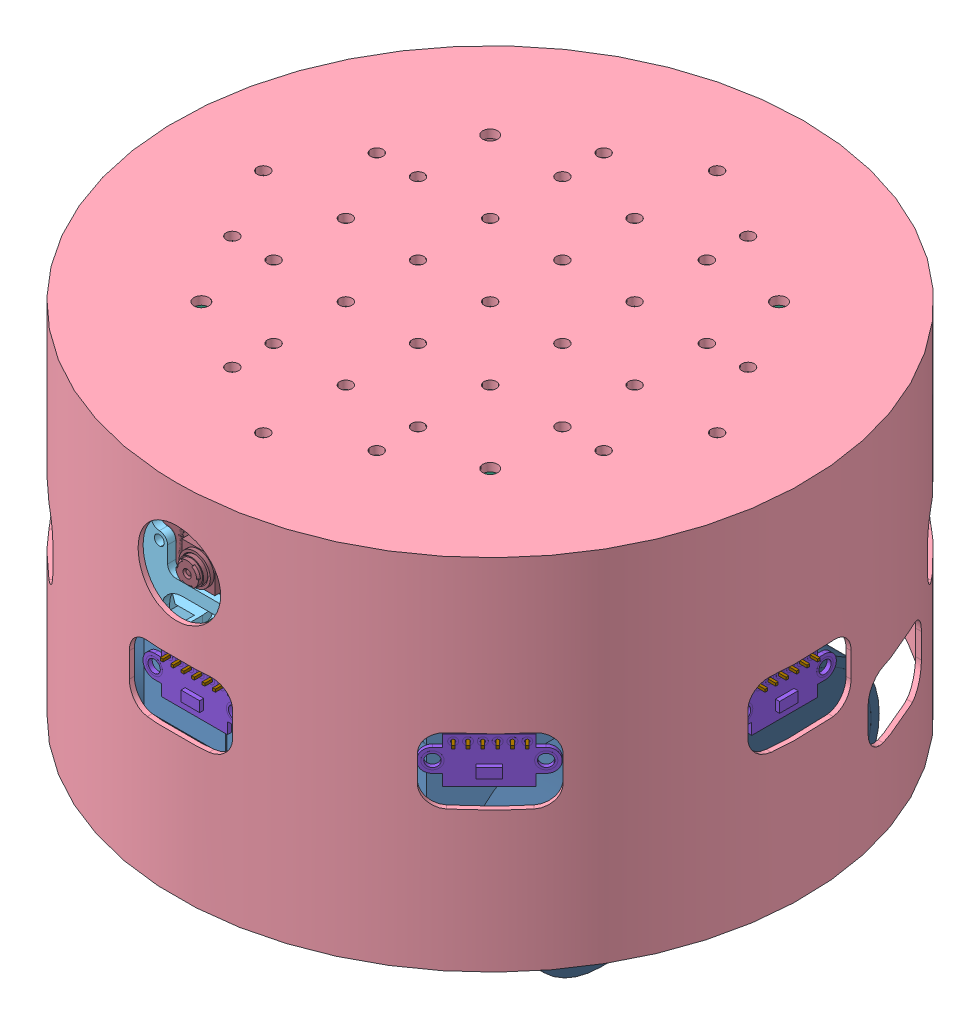
SolidWorks assembly affective_mobile_platform_ver_3, configuration Default. Lengths in mm.
Overall size (152 102.25 152).
598 component instances, 23 part files, 172 mates.
Components (placement in the parent):
- main_case-1: main_case [Default] at (56.0336 74.2064 51.1354) size (80.9 34.8 115.4)
- motor_holder-1: motor_holder [Default] at (56.0336 51.1064 74.8354) x (0 0 -1) z (-1 0 0) size (28 15 80.9)
- wheel_holder-1: wheel_holder [Default] at (74.0836 50.1064 122.8354) x (0 -1 0) z (0 0 1) size (14 20 27)
- wheel_holder-2: wheel_holder [Default] at (37.9836 50.1064 122.8354) x (0 -1 0) z (0 0 -1) size (14 20 27)
- power_bank-2: power_bank [Default] at (56.0336 72.6064 146.6354) x (-1 0 0) z (0 0 -1) size (66.5 23 95.6)
- 2nd_layer-1: 2nd_layer [Default] at (56.0336 89.3064 98.8354) size (130 1.6 130)
- H254_90deg_6pin-9: H254_90deg_6pin [Default] at (61.1135 93.4464 158.4354) x (-0.000003 0 1) z (1 -0.000004 0.000003) size (10.36 6.14 15.24)
  - H254_90deg_3pin-1: H254_90deg_3pin [Default] at origin size (10.36 6.14 7.62)
    - FrameAndPin_H254_90deg-1: FrameAndPin_H254_90deg [Default] at origin size (10.36 6.14 2.54)
      - frame_H254-1: frame_H254 [Default] at origin size (8.4 2.54 2.54)
      - pin-90deg-1: pin-90deg [Default] at (-0.0461 1.2682 1.27) x (0 0 -1) z (0.999998 -0.002105 0) size (1.95 5.07 7.58)
    - FrameAndPin_H254_90deg-2: FrameAndPin_H254_90deg [Default] at (0 0 -2.54) size (10.36 6.14 2.54)
      - frame_H254-1: frame_H254 [Default] at origin size (8.4 2.54 2.54)
      - pin-90deg-1: pin-90deg [Default] at (-0.0461 1.2682 1.27) x (0 0 -1) z (0.999998 -0.002105 0) size (1.95 5.07 7.58)
    - FrameAndPin_H254_90deg-4: FrameAndPin_H254_90deg [Default] at (0 0 -5.08) size (10.36 6.14 2.54)
      - frame_H254-1: frame_H254 [Default] at origin size (8.4 2.54 2.54)
      - pin-90deg-1: pin-90deg [Default] at (-0.0461 1.2682 1.27) x (0 0 -1) z (0.999998 -0.002105 0) size (1.95 5.07 7.58)
  - H254_90deg_3pin-2: H254_90deg_3pin [Default] at (0 0 -7.62) size (10.36 6.14 7.62)
    - FrameAndPin_H254_90deg-1: FrameAndPin_H254_90deg [Default] at origin size (10.36 6.14 2.54)
      - frame_H254-1: frame_H254 [Default] at origin size (8.4 2.54 2.54)
      - pin-90deg-1: pin-90deg [Default] at (-0.0461 1.2682 1.27) x (0 0 -1) z (0.999998 -0.002105 0) size (1.95 5.07 7.58)
    - FrameAndPin_H254_90deg-2: FrameAndPin_H254_90deg [Default] at (0 0 -2.54) size (10.36 6.14 2.54)
      - frame_H254-1: frame_H254 [Default] at origin size (8.4 2.54 2.54)
      - pin-90deg-1: pin-90deg [Default] at (-0.0461 1.2682 1.27) x (0 0 -1) z (0.999998 -0.002105 0) size (1.95 5.07 7.58)
    - FrameAndPin_H254_90deg-4: FrameAndPin_H254_90deg [Default] at (0 0 -5.08) size (10.36 6.14 2.54)
      - frame_H254-1: frame_H254 [Default] at origin size (8.4 2.54 2.54)
      - pin-90deg-1: pin-90deg [Default] at (-0.0461 1.2682 1.27) x (0 0 -1) z (0.999998 -0.002105 0) size (1.95 5.07 7.58)
- vl53l0x-9: vl53l0x [Default] at (55.8835 88.1764 169.3753) x (-1 0.000004 -0.000003) z (0.000004 1 0) size (25 11.3 11)
  - vl53l0x_PCB-1: vl53l0x_PCB [Default] at origin size (25 3 11)
  - pin_header-1: pin_header [Default] at (-6.5 -2.54 4) size (2.54 11.3 2.54)
  - pin_header-2: pin_header [Default] at (-3.96 -2.54 4) size (2.54 11.3 2.54)
  - pin_header-3: pin_header [Default] at (-1.42 -2.54 4) size (2.54 11.3 2.54)
  - pin_header-4: pin_header [Default] at (1.12 -2.54 4) size (2.54 11.3 2.54)
  - pin_header-5: pin_header [Default] at (3.66 -2.54 4) size (2.54 11.3 2.54)
  - pin_header-6: pin_header [Default] at (6.2 -2.54 4) size (2.54 11.3 2.54)
- wheels-1: wheels [Default] at (92.2336 51.1064 98.8354) x (0 0 -1) z (1 0 0) size (87 39 14.6)
- wheels-2: wheels [Default] at (19.8336 51.1064 98.8354) x (0 0 1) z (-1 0 0) size (87 39 14.6)
- spacer-2: spacer [Default] at (31.5336 90.9064 137.7975) x (0.77891 0 -0.627136) z (0.627136 0 0.77891) size (6.3 21 7.27)
- spacer-4: spacer [Default] at (80.5336 90.9064 79.7975) x (0 0 -1) z (1 0 0) size (6.3 21 7.27)
- spacer-5: spacer [Default] at (31.5336 90.9064 79.7975) x (0 0 1) z (-1 0 0) size (6.3 21 7.27)
- 1st_layer-1: 1st_layer [Default] at (37.9836 51.1064 122.8354) x (0 0 1) z (0 -1 0) size (65.3 46.5 2.57)
- vl53l0x-24: vl53l0x [Default] at (105.8067 88.1764 148.8208) x (-0.707109 0.000004 0.707104) z (0.000003 1 -0.000003) size (25 11.3 11)
  - vl53l0x_PCB-1: vl53l0x_PCB [Default] at origin size (25 3 11)
  - pin_header-1: pin_header [Default] at (-6.5 -2.54 4) size (2.54 11.3 2.54)
  - pin_header-2: pin_header [Default] at (-3.96 -2.54 4) size (2.54 11.3 2.54)
  - pin_header-3: pin_header [Default] at (-1.42 -2.54 4) size (2.54 11.3 2.54)
  - pin_header-4: pin_header [Default] at (1.12 -2.54 4) size (2.54 11.3 2.54)
  - pin_header-5: pin_header [Default] at (3.66 -2.54 4) size (2.54 11.3 2.54)
  - pin_header-6: pin_header [Default] at (6.2 -2.54 4) size (2.54 11.3 2.54)
- vl53l0x-25: vl53l0x [Default] at (126.5735 88.1764 98.9854) x (-0.000003 0.000004 1) z (0 1 -0.000004) size (25 11.3 11)
  - vl53l0x_PCB-1: vl53l0x_PCB [Default] at origin size (25 3 11)
  - pin_header-1: pin_header [Default] at (-6.5 -2.54 4) size (2.54 11.3 2.54)
  - pin_header-2: pin_header [Default] at (-3.96 -2.54 4) size (2.54 11.3 2.54)
  - pin_header-3: pin_header [Default] at (-1.42 -2.54 4) size (2.54 11.3 2.54)
  - pin_header-4: pin_header [Default] at (1.12 -2.54 4) size (2.54 11.3 2.54)
  - pin_header-5: pin_header [Default] at (3.66 -2.54 4) size (2.54 11.3 2.54)
  - pin_header-6: pin_header [Default] at (6.2 -2.54 4) size (2.54 11.3 2.54)
- vl53l0x-26: vl53l0x [Default] at (106.019 88.1764 49.0622) x (0.707104 0.000004 0.707109) z (-0.000003 1 -0.000003) size (25 11.3 11)
  - vl53l0x_PCB-1: vl53l0x_PCB [Default] at origin size (25 3 11)
  - pin_header-1: pin_header [Default] at (-6.5 -2.54 4) size (2.54 11.3 2.54)
  - pin_header-2: pin_header [Default] at (-3.96 -2.54 4) size (2.54 11.3 2.54)
  - pin_header-3: pin_header [Default] at (-1.42 -2.54 4) size (2.54 11.3 2.54)
  - pin_header-4: pin_header [Default] at (1.12 -2.54 4) size (2.54 11.3 2.54)
  - pin_header-5: pin_header [Default] at (3.66 -2.54 4) size (2.54 11.3 2.54)
  - pin_header-6: pin_header [Default] at (6.2 -2.54 4) size (2.54 11.3 2.54)
- vl53l0x-27: vl53l0x [Default] at (56.1836 88.1764 28.2954) x (1 0.000004 0.000003) z (-0.000004 1 0) size (25 11.3 11)
  - vl53l0x_PCB-1: vl53l0x_PCB [Default] at origin size (25 3 11)
  - pin_header-1: pin_header [Default] at (-6.5 -2.54 4) size (2.54 11.3 2.54)
  - pin_header-2: pin_header [Default] at (-3.96 -2.54 4) size (2.54 11.3 2.54)
  - pin_header-3: pin_header [Default] at (-1.42 -2.54 4) size (2.54 11.3 2.54)
  - pin_header-4: pin_header [Default] at (1.12 -2.54 4) size (2.54 11.3 2.54)
  - pin_header-5: pin_header [Default] at (3.66 -2.54 4) size (2.54 11.3 2.54)
  - pin_header-6: pin_header [Default] at (6.2 -2.54 4) size (2.54 11.3 2.54)
- vl53l0x-28: vl53l0x [Default] at (6.2604 88.1764 48.85) x (0.707109 0.000004 -0.707104) z (-0.000003 1 0.000003) size (25 11.3 11)
  - vl53l0x_PCB-1: vl53l0x_PCB [Default] at origin size (25 3 11)
  - pin_header-1: pin_header [Default] at (-6.5 -2.54 4) size (2.54 11.3 2.54)
  - pin_header-2: pin_header [Default] at (-3.96 -2.54 4) size (2.54 11.3 2.54)
  - pin_header-3: pin_header [Default] at (-1.42 -2.54 4) size (2.54 11.3 2.54)
  - pin_header-4: pin_header [Default] at (1.12 -2.54 4) size (2.54 11.3 2.54)
  - pin_header-5: pin_header [Default] at (3.66 -2.54 4) size (2.54 11.3 2.54)
  - pin_header-6: pin_header [Default] at (6.2 -2.54 4) size (2.54 11.3 2.54)
- vl53l0x-29: vl53l0x [Default] at (-14.5064 88.1764 98.6853) x (0.000003 0.000004 -1) z (0 1 0.000004) size (25 11.3 11)
  - vl53l0x_PCB-1: vl53l0x_PCB [Default] at origin size (25 3 11)
  - pin_header-1: pin_header [Default] at (-6.5 -2.54 4) size (2.54 11.3 2.54)
  - pin_header-2: pin_header [Default] at (-3.96 -2.54 4) size (2.54 11.3 2.54)
  - pin_header-3: pin_header [Default] at (-1.42 -2.54 4) size (2.54 11.3 2.54)
  - pin_header-4: pin_header [Default] at (1.12 -2.54 4) size (2.54 11.3 2.54)
  - pin_header-5: pin_header [Default] at (3.66 -2.54 4) size (2.54 11.3 2.54)
  - pin_header-6: pin_header [Default] at (6.2 -2.54 4) size (2.54 11.3 2.54)
- vl53l0x-30: vl53l0x [Default] at (6.0481 88.1764 148.6086) x (-0.707104 0.000004 -0.707109) z (0.000003 1 0.000003) size (25 11.3 11)
  - vl53l0x_PCB-1: vl53l0x_PCB [Default] at origin size (25 3 11)
  - pin_header-1: pin_header [Default] at (-6.5 -2.54 4) size (2.54 11.3 2.54)
  - pin_header-2: pin_header [Default] at (-3.96 -2.54 4) size (2.54 11.3 2.54)
  - pin_header-3: pin_header [Default] at (-1.42 -2.54 4) size (2.54 11.3 2.54)
  - pin_header-4: pin_header [Default] at (1.12 -2.54 4) size (2.54 11.3 2.54)
  - pin_header-5: pin_header [Default] at (3.66 -2.54 4) size (2.54 11.3 2.54)
  - pin_header-6: pin_header [Default] at (6.2 -2.54 4) size (2.54 11.3 2.54)
- H254_90deg_6pin-24: H254_90deg_6pin [Default] at (101.7692 93.4464 137.3868) x (0.707104 0 0.707109) z (0.707109 -0.000004 -0.707104) size (10.36 6.14 15.24)
  - H254_90deg_3pin-1: H254_90deg_3pin [Default] at origin size (10.36 6.14 7.62)
    - FrameAndPin_H254_90deg-1: FrameAndPin_H254_90deg [Default] at origin size (10.36 6.14 2.54)
      - frame_H254-1: frame_H254 [Default] at origin size (8.4 2.54 2.54)
      - pin-90deg-1: pin-90deg [Default] at (-0.0461 1.2682 1.27) x (0 0 -1) z (0.999998 -0.002105 0) size (1.95 5.07 7.58)
    - FrameAndPin_H254_90deg-2: FrameAndPin_H254_90deg [Default] at (0 0 -2.54) size (10.36 6.14 2.54)
      - frame_H254-1: frame_H254 [Default] at origin size (8.4 2.54 2.54)
      - pin-90deg-1: pin-90deg [Default] at (-0.0461 1.2682 1.27) x (0 0 -1) z (0.999998 -0.002105 0) size (1.95 5.07 7.58)
    - FrameAndPin_H254_90deg-4: FrameAndPin_H254_90deg [Default] at (0 0 -5.08) size (10.36 6.14 2.54)
      - frame_H254-1: frame_H254 [Default] at origin size (8.4 2.54 2.54)
      - pin-90deg-1: pin-90deg [Default] at (-0.0461 1.2682 1.27) x (0 0 -1) z (0.999998 -0.002105 0) size (1.95 5.07 7.58)
  - H254_90deg_3pin-2: H254_90deg_3pin [Default] at (0 0 -7.62) size (10.36 6.14 7.62)
    - FrameAndPin_H254_90deg-1: FrameAndPin_H254_90deg [Default] at origin size (10.36 6.14 2.54)
      - frame_H254-1: frame_H254 [Default] at origin size (8.4 2.54 2.54)
      - pin-90deg-1: pin-90deg [Default] at (-0.0461 1.2682 1.27) x (0 0 -1) z (0.999998 -0.002105 0) size (1.95 5.07 7.58)
    - FrameAndPin_H254_90deg-2: FrameAndPin_H254_90deg [Default] at (0 0 -2.54) size (10.36 6.14 2.54)
      - frame_H254-1: frame_H254 [Default] at origin size (8.4 2.54 2.54)
      - pin-90deg-1: pin-90deg [Default] at (-0.0461 1.2682 1.27) x (0 0 -1) z (0.999998 -0.002105 0) size (1.95 5.07 7.58)
    - FrameAndPin_H254_90deg-4: FrameAndPin_H254_90deg [Default] at (0 0 -5.08) size (10.36 6.14 2.54)
      - frame_H254-1: frame_H254 [Default] at origin size (8.4 2.54 2.54)
      - pin-90deg-1: pin-90deg [Default] at (-0.0461 1.2682 1.27) x (0 0 -1) z (0.999998 -0.002105 0) size (1.95 5.07 7.58)
- H254_90deg_6pin-25: H254_90deg_6pin [Default] at (115.6336 93.4464 93.7554) x (1 0 0.000003) z (0.000003 -0.000004 -1) size (10.36 6.14 15.24)
  - H254_90deg_3pin-1: H254_90deg_3pin [Default] at origin size (10.36 6.14 7.62)
    - FrameAndPin_H254_90deg-1: FrameAndPin_H254_90deg [Default] at origin size (10.36 6.14 2.54)
      - frame_H254-1: frame_H254 [Default] at origin size (8.4 2.54 2.54)
      - pin-90deg-1: pin-90deg [Default] at (-0.0461 1.2682 1.27) x (0 0 -1) z (0.999998 -0.002105 0) size (1.95 5.07 7.58)
    - FrameAndPin_H254_90deg-2: FrameAndPin_H254_90deg [Default] at (0 0 -2.54) size (10.36 6.14 2.54)
      - frame_H254-1: frame_H254 [Default] at origin size (8.4 2.54 2.54)
      - pin-90deg-1: pin-90deg [Default] at (-0.0461 1.2682 1.27) x (0 0 -1) z (0.999998 -0.002105 0) size (1.95 5.07 7.58)
    - FrameAndPin_H254_90deg-4: FrameAndPin_H254_90deg [Default] at (0 0 -5.08) size (10.36 6.14 2.54)
      - frame_H254-1: frame_H254 [Default] at origin size (8.4 2.54 2.54)
      - pin-90deg-1: pin-90deg [Default] at (-0.0461 1.2682 1.27) x (0 0 -1) z (0.999998 -0.002105 0) size (1.95 5.07 7.58)
  - H254_90deg_3pin-2: H254_90deg_3pin [Default] at (0 0 -7.62) size (10.36 6.14 7.62)
    - FrameAndPin_H254_90deg-1: FrameAndPin_H254_90deg [Default] at origin size (10.36 6.14 2.54)
      - frame_H254-1: frame_H254 [Default] at origin size (8.4 2.54 2.54)
      - pin-90deg-1: pin-90deg [Default] at (-0.0461 1.2682 1.27) x (0 0 -1) z (0.999998 -0.002105 0) size (1.95 5.07 7.58)
    - FrameAndPin_H254_90deg-2: FrameAndPin_H254_90deg [Default] at (0 0 -2.54) size (10.36 6.14 2.54)
      - frame_H254-1: frame_H254 [Default] at origin size (8.4 2.54 2.54)
      - pin-90deg-1: pin-90deg [Default] at (-0.0461 1.2682 1.27) x (0 0 -1) z (0.999998 -0.002105 0) size (1.95 5.07 7.58)
    - FrameAndPin_H254_90deg-4: FrameAndPin_H254_90deg [Default] at (0 0 -5.08) size (10.36 6.14 2.54)
      - frame_H254-1: frame_H254 [Default] at origin size (8.4 2.54 2.54)
      - pin-90deg-1: pin-90deg [Default] at (-0.0461 1.2682 1.27) x (0 0 -1) z (0.999998 -0.002105 0) size (1.95 5.07 7.58)
- H254_90deg_6pin-26: H254_90deg_6pin [Default] at (94.585 93.4464 53.0997) x (0.707109 0 -0.707104) z (-0.707104 -0.000004 -0.707109) size (10.36 6.14 15.24)
  - H254_90deg_3pin-1: H254_90deg_3pin [Default] at origin size (10.36 6.14 7.62)
    - FrameAndPin_H254_90deg-1: FrameAndPin_H254_90deg [Default] at origin size (10.36 6.14 2.54)
      - frame_H254-1: frame_H254 [Default] at origin size (8.4 2.54 2.54)
      - pin-90deg-1: pin-90deg [Default] at (-0.0461 1.2682 1.27) x (0 0 -1) z (0.999998 -0.002105 0) size (1.95 5.07 7.58)
    - FrameAndPin_H254_90deg-2: FrameAndPin_H254_90deg [Default] at (0 0 -2.54) size (10.36 6.14 2.54)
      - frame_H254-1: frame_H254 [Default] at origin size (8.4 2.54 2.54)
      - pin-90deg-1: pin-90deg [Default] at (-0.0461 1.2682 1.27) x (0 0 -1) z (0.999998 -0.002105 0) size (1.95 5.07 7.58)
    - FrameAndPin_H254_90deg-4: FrameAndPin_H254_90deg [Default] at (0 0 -5.08) size (10.36 6.14 2.54)
      - frame_H254-1: frame_H254 [Default] at origin size (8.4 2.54 2.54)
      - pin-90deg-1: pin-90deg [Default] at (-0.0461 1.2682 1.27) x (0 0 -1) z (0.999998 -0.002105 0) size (1.95 5.07 7.58)
  - H254_90deg_3pin-2: H254_90deg_3pin [Default] at (0 0 -7.62) size (10.36 6.14 7.62)
    - FrameAndPin_H254_90deg-1: FrameAndPin_H254_90deg [Default] at origin size (10.36 6.14 2.54)
      - frame_H254-1: frame_H254 [Default] at origin size (8.4 2.54 2.54)
      - pin-90deg-1: pin-90deg [Default] at (-0.0461 1.2682 1.27) x (0 0 -1) z (0.999998 -0.002105 0) size (1.95 5.07 7.58)
    - FrameAndPin_H254_90deg-2: FrameAndPin_H254_90deg [Default] at (0 0 -2.54) size (10.36 6.14 2.54)
      - frame_H254-1: frame_H254 [Default] at origin size (8.4 2.54 2.54)
      - pin-90deg-1: pin-90deg [Default] at (-0.0461 1.2682 1.27) x (0 0 -1) z (0.999998 -0.002105 0) size (1.95 5.07 7.58)
    - FrameAndPin_H254_90deg-4: FrameAndPin_H254_90deg [Default] at (0 0 -5.08) size (10.36 6.14 2.54)
      - frame_H254-1: frame_H254 [Default] at origin size (8.4 2.54 2.54)
      - pin-90deg-1: pin-90deg [Default] at (-0.0461 1.2682 1.27) x (0 0 -1) z (0.999998 -0.002105 0) size (1.95 5.07 7.58)
- H254_90deg_6pin-27: H254_90deg_6pin [Default] at (50.9536 93.4464 39.2354) x (0.000003 0 -1) z (-1 -0.000004 -0.000003) size (10.36 6.14 15.24)
  - H254_90deg_3pin-1: H254_90deg_3pin [Default] at origin size (10.36 6.14 7.62)
    - FrameAndPin_H254_90deg-1: FrameAndPin_H254_90deg [Default] at origin size (10.36 6.14 2.54)
      - frame_H254-1: frame_H254 [Default] at origin size (8.4 2.54 2.54)
      - pin-90deg-1: pin-90deg [Default] at (-0.0461 1.2682 1.27) x (0 0 -1) z (0.999998 -0.002105 0) size (1.95 5.07 7.58)
    - FrameAndPin_H254_90deg-2: FrameAndPin_H254_90deg [Default] at (0 0 -2.54) size (10.36 6.14 2.54)
      - frame_H254-1: frame_H254 [Default] at origin size (8.4 2.54 2.54)
      - pin-90deg-1: pin-90deg [Default] at (-0.0461 1.2682 1.27) x (0 0 -1) z (0.999998 -0.002105 0) size (1.95 5.07 7.58)
    - FrameAndPin_H254_90deg-4: FrameAndPin_H254_90deg [Default] at (0 0 -5.08) size (10.36 6.14 2.54)
      - frame_H254-1: frame_H254 [Default] at origin size (8.4 2.54 2.54)
      - pin-90deg-1: pin-90deg [Default] at (-0.0461 1.2682 1.27) x (0 0 -1) z (0.999998 -0.002105 0) size (1.95 5.07 7.58)
  - H254_90deg_3pin-2: H254_90deg_3pin [Default] at (0 0 -7.62) size (10.36 6.14 7.62)
    - FrameAndPin_H254_90deg-1: FrameAndPin_H254_90deg [Default] at origin size (10.36 6.14 2.54)
      - frame_H254-1: frame_H254 [Default] at origin size (8.4 2.54 2.54)
      - pin-90deg-1: pin-90deg [Default] at (-0.0461 1.2682 1.27) x (0 0 -1) z (0.999998 -0.002105 0) size (1.95 5.07 7.58)
    - FrameAndPin_H254_90deg-2: FrameAndPin_H254_90deg [Default] at (0 0 -2.54) size (10.36 6.14 2.54)
      - frame_H254-1: frame_H254 [Default] at origin size (8.4 2.54 2.54)
      - pin-90deg-1: pin-90deg [Default] at (-0.0461 1.2682 1.27) x (0 0 -1) z (0.999998 -0.002105 0) size (1.95 5.07 7.58)
    - FrameAndPin_H254_90deg-4: FrameAndPin_H254_90deg [Default] at (0 0 -5.08) size (10.36 6.14 2.54)
      - frame_H254-1: frame_H254 [Default] at origin size (8.4 2.54 2.54)
      - pin-90deg-1: pin-90deg [Default] at (-0.0461 1.2682 1.27) x (0 0 -1) z (0.999998 -0.002105 0) size (1.95 5.07 7.58)
- H254_90deg_6pin-28: H254_90deg_6pin [Default] at (10.2979 93.4464 60.2839) x (-0.707104 0 -0.707109) z (-0.707109 -0.000004 0.707104) size (10.36 6.14 15.24)
  - H254_90deg_3pin-1: H254_90deg_3pin [Default] at origin size (10.36 6.14 7.62)
    - FrameAndPin_H254_90deg-1: FrameAndPin_H254_90deg [Default] at origin size (10.36 6.14 2.54)
      - frame_H254-1: frame_H254 [Default] at origin size (8.4 2.54 2.54)
      - pin-90deg-1: pin-90deg [Default] at (-0.0461 1.2682 1.27) x (0 0 -1) z (0.999998 -0.002105 0) size (1.95 5.07 7.58)
    - FrameAndPin_H254_90deg-2: FrameAndPin_H254_90deg [Default] at (0 0 -2.54) size (10.36 6.14 2.54)
      - frame_H254-1: frame_H254 [Default] at origin size (8.4 2.54 2.54)
      - pin-90deg-1: pin-90deg [Default] at (-0.0461 1.2682 1.27) x (0 0 -1) z (0.999998 -0.002105 0) size (1.95 5.07 7.58)
    - FrameAndPin_H254_90deg-4: FrameAndPin_H254_90deg [Default] at (0 0 -5.08) size (10.36 6.14 2.54)
      - frame_H254-1: frame_H254 [Default] at origin size (8.4 2.54 2.54)
      - pin-90deg-1: pin-90deg [Default] at (-0.0461 1.2682 1.27) x (0 0 -1) z (0.999998 -0.002105 0) size (1.95 5.07 7.58)
  - H254_90deg_3pin-2: H254_90deg_3pin [Default] at (0 0 -7.62) size (10.36 6.14 7.62)
    - FrameAndPin_H254_90deg-1: FrameAndPin_H254_90deg [Default] at origin size (10.36 6.14 2.54)
      - frame_H254-1: frame_H254 [Default] at origin size (8.4 2.54 2.54)
      - pin-90deg-1: pin-90deg [Default] at (-0.0461 1.2682 1.27) x (0 0 -1) z (0.999998 -0.002105 0) size (1.95 5.07 7.58)
    - FrameAndPin_H254_90deg-2: FrameAndPin_H254_90deg [Default] at (0 0 -2.54) size (10.36 6.14 2.54)
      - frame_H254-1: frame_H254 [Default] at origin size (8.4 2.54 2.54)
      - pin-90deg-1: pin-90deg [Default] at (-0.0461 1.2682 1.27) x (0 0 -1) z (0.999998 -0.002105 0) size (1.95 5.07 7.58)
    - FrameAndPin_H254_90deg-4: FrameAndPin_H254_90deg [Default] at (0 0 -5.08) size (10.36 6.14 2.54)
      - frame_H254-1: frame_H254 [Default] at origin size (8.4 2.54 2.54)
      - pin-90deg-1: pin-90deg [Default] at (-0.0461 1.2682 1.27) x (0 0 -1) z (0.999998 -0.002105 0) size (1.95 5.07 7.58)
- H254_90deg_6pin-29: H254_90deg_6pin [Default] at (-3.5664 93.4464 103.9154) x (-1 0 -0.000003) z (-0.000003 -0.000004 1) size (10.36 6.14 15.24)
  - H254_90deg_3pin-1: H254_90deg_3pin [Default] at origin size (10.36 6.14 7.62)
    - FrameAndPin_H254_90deg-1: FrameAndPin_H254_90deg [Default] at origin size (10.36 6.14 2.54)
      - frame_H254-1: frame_H254 [Default] at origin size (8.4 2.54 2.54)
      - pin-90deg-1: pin-90deg [Default] at (-0.0461 1.2682 1.27) x (0 0 -1) z (0.999998 -0.002105 0) size (1.95 5.07 7.58)
    - FrameAndPin_H254_90deg-2: FrameAndPin_H254_90deg [Default] at (0 0 -2.54) size (10.36 6.14 2.54)
      - frame_H254-1: frame_H254 [Default] at origin size (8.4 2.54 2.54)
      - pin-90deg-1: pin-90deg [Default] at (-0.0461 1.2682 1.27) x (0 0 -1) z (0.999998 -0.002105 0) size (1.95 5.07 7.58)
    - FrameAndPin_H254_90deg-4: FrameAndPin_H254_90deg [Default] at (0 0 -5.08) size (10.36 6.14 2.54)
      - frame_H254-1: frame_H254 [Default] at origin size (8.4 2.54 2.54)
      - pin-90deg-1: pin-90deg [Default] at (-0.0461 1.2682 1.27) x (0 0 -1) z (0.999998 -0.002105 0) size (1.95 5.07 7.58)
  - H254_90deg_3pin-2: H254_90deg_3pin [Default] at (0 0 -7.62) size (10.36 6.14 7.62)
    - FrameAndPin_H254_90deg-1: FrameAndPin_H254_90deg [Default] at origin size (10.36 6.14 2.54)
      - frame_H254-1: frame_H254 [Default] at origin size (8.4 2.54 2.54)
      - pin-90deg-1: pin-90deg [Default] at (-0.0461 1.2682 1.27) x (0 0 -1) z (0.999998 -0.002105 0) size (1.95 5.07 7.58)
    - FrameAndPin_H254_90deg-2: FrameAndPin_H254_90deg [Default] at (0 0 -2.54) size (10.36 6.14 2.54)
      - frame_H254-1: frame_H254 [Default] at origin size (8.4 2.54 2.54)
      - pin-90deg-1: pin-90deg [Default] at (-0.0461 1.2682 1.27) x (0 0 -1) z (0.999998 -0.002105 0) size (1.95 5.07 7.58)
    - FrameAndPin_H254_90deg-4: FrameAndPin_H254_90deg [Default] at (0 0 -5.08) size (10.36 6.14 2.54)
      - frame_H254-1: frame_H254 [Default] at origin size (8.4 2.54 2.54)
      - pin-90deg-1: pin-90deg [Default] at (-0.0461 1.2682 1.27) x (0 0 -1) z (0.999998 -0.002105 0) size (1.95 5.07 7.58)
- H254_90deg_6pin-30: H254_90deg_6pin [Default] at (17.4821 93.4464 144.571) x (-0.707109 0 0.707104) z (0.707104 -0.000004 0.707109) size (10.36 6.14 15.24)
  - H254_90deg_3pin-1: H254_90deg_3pin [Default] at origin size (10.36 6.14 7.62)
    - FrameAndPin_H254_90deg-1: FrameAndPin_H254_90deg [Default] at origin size (10.36 6.14 2.54)
      - frame_H254-1: frame_H254 [Default] at origin size (8.4 2.54 2.54)
      - pin-90deg-1: pin-90deg [Default] at (-0.0461 1.2682 1.27) x (0 0 -1) z (0.999998 -0.002105 0) size (1.95 5.07 7.58)
    - FrameAndPin_H254_90deg-2: FrameAndPin_H254_90deg [Default] at (0 0 -2.54) size (10.36 6.14 2.54)
      - frame_H254-1: frame_H254 [Default] at origin size (8.4 2.54 2.54)
      - pin-90deg-1: pin-90deg [Default] at (-0.0461 1.2682 1.27) x (0 0 -1) z (0.999998 -0.002105 0) size (1.95 5.07 7.58)
    - FrameAndPin_H254_90deg-4: FrameAndPin_H254_90deg [Default] at (0 0 -5.08) size (10.36 6.14 2.54)
      - frame_H254-1: frame_H254 [Default] at origin size (8.4 2.54 2.54)
      - pin-90deg-1: pin-90deg [Default] at (-0.0461 1.2682 1.27) x (0 0 -1) z (0.999998 -0.002105 0) size (1.95 5.07 7.58)
  - H254_90deg_3pin-2: H254_90deg_3pin [Default] at (0 0 -7.62) size (10.36 6.14 7.62)
    - FrameAndPin_H254_90deg-1: FrameAndPin_H254_90deg [Default] at origin size (10.36 6.14 2.54)
      - frame_H254-1: frame_H254 [Default] at origin size (8.4 2.54 2.54)
      - pin-90deg-1: pin-90deg [Default] at (-0.0461 1.2682 1.27) x (0 0 -1) z (0.999998 -0.002105 0) size (1.95 5.07 7.58)
    - FrameAndPin_H254_90deg-2: FrameAndPin_H254_90deg [Default] at (0 0 -2.54) size (10.36 6.14 2.54)
      - frame_H254-1: frame_H254 [Default] at origin size (8.4 2.54 2.54)
      - pin-90deg-1: pin-90deg [Default] at (-0.0461 1.2682 1.27) x (0 0 -1) z (0.999998 -0.002105 0) size (1.95 5.07 7.58)
    - FrameAndPin_H254_90deg-4: FrameAndPin_H254_90deg [Default] at (0 0 -5.08) size (10.36 6.14 2.54)
      - frame_H254-1: frame_H254 [Default] at origin size (8.4 2.54 2.54)
      - pin-90deg-1: pin-90deg [Default] at (-0.0461 1.2682 1.27) x (0 0 -1) z (0.999998 -0.002105 0) size (1.95 5.07 7.58)
- camera-1: camera [Default] at (56.1278 115.9111 165.5354) x (0 1 0) z (0 0 1) size (23.86 25 9.96)
- raspberryPi3B-1: raspberryPi3B [Detailed] at (56.0336 107.2064 98.7975) x (0 0 -1) z (0 -1 0) size (87.05 58.5 19.05)
- spacer-8: spacer [Default] at (80.5336 90.9064 137.7975) x (0.77891 0 -0.627136) z (0.627136 0 0.77891) size (6.3 21 7.27)
- 3rd_layer-1: 3rd_layer [Default] at (56.0336 115.2592 98.8354) x (-1 0 0) z (0 1 0) size (130 109 1.6)
- Header_1x20pin-1: Header_1x20pin [Default] at (105.5636 90.9064 122.1244) size (2.54 10.59 50.8)
  - header-1: header [Default] at origin size (2.54 10.59 2.54)
    - header-1: header [Default] at origin size (2.54 8.5 2.54)
    - pin-1: pin [Default] at (-1.4 0 0) size (0.4 10 1.99)
  - header-2: header [Default] at (0 0 -2.54) size (2.54 10.59 2.54)
    - header-1: header [Default] at origin size (2.54 8.5 2.54)
    - pin-1: pin [Default] at (-1.4 0 0) size (0.4 10 1.99)
  - header-3: header [Default] at (0 0 -5.08) size (2.54 10.59 2.54)
    - header-1: header [Default] at origin size (2.54 8.5 2.54)
    - pin-1: pin [Default] at (-1.4 0 0) size (0.4 10 1.99)
  - header-4: header [Default] at (0 0 -7.62) size (2.54 10.59 2.54)
    - header-1: header [Default] at origin size (2.54 8.5 2.54)
    - pin-1: pin [Default] at (-1.4 0 0) size (0.4 10 1.99)
  - header-5: header [Default] at (0 0 -10.16) size (2.54 10.59 2.54)
    - header-1: header [Default] at origin size (2.54 8.5 2.54)
    - pin-1: pin [Default] at (-1.4 0 0) size (0.4 10 1.99)
  - header-6: header [Default] at (0 0 -12.7) size (2.54 10.59 2.54)
    - header-1: header [Default] at origin size (2.54 8.5 2.54)
    - pin-1: pin [Default] at (-1.4 0 0) size (0.4 10 1.99)
  - header-7: header [Default] at (0 0 -15.24) size (2.54 10.59 2.54)
    - header-1: header [Default] at origin size (2.54 8.5 2.54)
    - pin-1: pin [Default] at (-1.4 0 0) size (0.4 10 1.99)
  - header-8: header [Default] at (0 0 -17.78) size (2.54 10.59 2.54)
    - header-1: header [Default] at origin size (2.54 8.5 2.54)
    - pin-1: pin [Default] at (-1.4 0 0) size (0.4 10 1.99)
  - header-9: header [Default] at (0 0 -20.32) size (2.54 10.59 2.54)
    - header-1: header [Default] at origin size (2.54 8.5 2.54)
    - pin-1: pin [Default] at (-1.4 0 0) size (0.4 10 1.99)
  - header-10: header [Default] at (0 0 -22.86) size (2.54 10.59 2.54)
    - header-1: header [Default] at origin size (2.54 8.5 2.54)
    - pin-1: pin [Default] at (-1.4 0 0) size (0.4 10 1.99)
  - header-11: header [Default] at (0 0 -25.4) size (2.54 10.59 2.54)
    - header-1: header [Default] at origin size (2.54 8.5 2.54)
    - pin-1: pin [Default] at (-1.4 0 0) size (0.4 10 1.99)
  - header-12: header [Default] at (0 0 -27.94) size (2.54 10.59 2.54)
    - header-1: header [Default] at origin size (2.54 8.5 2.54)
    - pin-1: pin [Default] at (-1.4 0 0) size (0.4 10 1.99)
  - header-13: header [Default] at (0 0 -30.48) size (2.54 10.59 2.54)
    - header-1: header [Default] at origin size (2.54 8.5 2.54)
    - pin-1: pin [Default] at (-1.4 0 0) size (0.4 10 1.99)
  - header-14: header [Default] at (0 0 -33.02) size (2.54 10.59 2.54)
    - header-1: header [Default] at origin size (2.54 8.5 2.54)
    - pin-1: pin [Default] at (-1.4 0 0) size (0.4 10 1.99)
  - header-15: header [Default] at (0 0 -35.56) size (2.54 10.59 2.54)
    - header-1: header [Default] at origin size (2.54 8.5 2.54)
    - pin-1: pin [Default] at (-1.4 0 0) size (0.4 10 1.99)
  - header-16: header [Default] at (0 0 -38.1) size (2.54 10.59 2.54)
    - header-1: header [Default] at origin size (2.54 8.5 2.54)
    - pin-1: pin [Default] at (-1.4 0 0) size (0.4 10 1.99)
  - header-17: header [Default] at (0 0 -40.64) size (2.54 10.59 2.54)
    - header-1: header [Default] at origin size (2.54 8.5 2.54)
    - pin-1: pin [Default] at (-1.4 0 0) size (0.4 10 1.99)
  - header-18: header [Default] at (0 0 -43.18) size (2.54 10.59 2.54)
    - header-1: header [Default] at origin size (2.54 8.5 2.54)
    - pin-1: pin [Default] at (-1.4 0 0) size (0.4 10 1.99)
  - header-19: header [Default] at (0 0 -45.72) size (2.54 10.59 2.54)
    - header-1: header [Default] at origin size (2.54 8.5 2.54)
    - pin-1: pin [Default] at (-1.4 0 0) size (0.4 10 1.99)
  - header-20: header [Default] at (0 0 -48.26) size (2.54 10.59 2.54)
    - header-1: header [Default] at origin size (2.54 8.5 2.54)
    - pin-1: pin [Default] at (-1.4 0 0) size (0.4 10 1.99)
- Header_1x20pin-2: Header_1x20pin [Default] at (9.0436 90.9064 122.1244) size (2.54 10.59 50.8)
  - header-1: header [Default] at origin size (2.54 10.59 2.54)
    - header-1: header [Default] at origin size (2.54 8.5 2.54)
    - pin-1: pin [Default] at (-1.4 0 0) size (0.4 10 1.99)
  - header-2: header [Default] at (0 0 -2.54) size (2.54 10.59 2.54)
    - header-1: header [Default] at origin size (2.54 8.5 2.54)
    - pin-1: pin [Default] at (-1.4 0 0) size (0.4 10 1.99)
  - header-3: header [Default] at (0 0 -5.08) size (2.54 10.59 2.54)
    - header-1: header [Default] at origin size (2.54 8.5 2.54)
    - pin-1: pin [Default] at (-1.4 0 0) size (0.4 10 1.99)
  - header-4: header [Default] at (0 0 -7.62) size (2.54 10.59 2.54)
    - header-1: header [Default] at origin size (2.54 8.5 2.54)
    - pin-1: pin [Default] at (-1.4 0 0) size (0.4 10 1.99)
  - header-5: header [Default] at (0 0 -10.16) size (2.54 10.59 2.54)
    - header-1: header [Default] at origin size (2.54 8.5 2.54)
    - pin-1: pin [Default] at (-1.4 0 0) size (0.4 10 1.99)
  - header-6: header [Default] at (0 0 -12.7) size (2.54 10.59 2.54)
    - header-1: header [Default] at origin size (2.54 8.5 2.54)
    - pin-1: pin [Default] at (-1.4 0 0) size (0.4 10 1.99)
  - header-7: header [Default] at (0 0 -15.24) size (2.54 10.59 2.54)
    - header-1: header [Default] at origin size (2.54 8.5 2.54)
    - pin-1: pin [Default] at (-1.4 0 0) size (0.4 10 1.99)
  - header-8: header [Default] at (0 0 -17.78) size (2.54 10.59 2.54)
    - header-1: header [Default] at origin size (2.54 8.5 2.54)
    - pin-1: pin [Default] at (-1.4 0 0) size (0.4 10 1.99)
  - header-9: header [Default] at (0 0 -20.32) size (2.54 10.59 2.54)
    - header-1: header [Default] at origin size (2.54 8.5 2.54)
    - pin-1: pin [Default] at (-1.4 0 0) size (0.4 10 1.99)
  - header-10: header [Default] at (0 0 -22.86) size (2.54 10.59 2.54)
    - header-1: header [Default] at origin size (2.54 8.5 2.54)
    - pin-1: pin [Default] at (-1.4 0 0) size (0.4 10 1.99)
  - header-11: header [Default] at (0 0 -25.4) size (2.54 10.59 2.54)
    - header-1: header [Default] at origin size (2.54 8.5 2.54)
    - pin-1: pin [Default] at (-1.4 0 0) size (0.4 10 1.99)
  - header-12: header [Default] at (0 0 -27.94) size (2.54 10.59 2.54)
    - header-1: header [Default] at origin size (2.54 8.5 2.54)
    - pin-1: pin [Default] at (-1.4 0 0) size (0.4 10 1.99)
  - header-13: header [Default] at (0 0 -30.48) size (2.54 10.59 2.54)
    - header-1: header [Default] at origin size (2.54 8.5 2.54)
    - pin-1: pin [Default] at (-1.4 0 0) size (0.4 10 1.99)
  - header-14: header [Default] at (0 0 -33.02) size (2.54 10.59 2.54)
    - header-1: header [Default] at origin size (2.54 8.5 2.54)
    - pin-1: pin [Default] at (-1.4 0 0) size (0.4 10 1.99)
  - header-15: header [Default] at (0 0 -35.56) size (2.54 10.59 2.54)
    - header-1: header [Default] at origin size (2.54 8.5 2.54)
    - pin-1: pin [Default] at (-1.4 0 0) size (0.4 10 1.99)
  - header-16: header [Default] at (0 0 -38.1) size (2.54 10.59 2.54)
    - header-1: header [Default] at origin size (2.54 8.5 2.54)
    - pin-1: pin [Default] at (-1.4 0 0) size (0.4 10 1.99)
  - header-17: header [Default] at (0 0 -40.64) size (2.54 10.59 2.54)
    - header-1: header [Default] at origin size (2.54 8.5 2.54)
    - pin-1: pin [Default] at (-1.4 0 0) size (0.4 10 1.99)
  - header-18: header [Default] at (0 0 -43.18) size (2.54 10.59 2.54)
    - header-1: header [Default] at origin size (2.54 8.5 2.54)
    - pin-1: pin [Default] at (-1.4 0 0) size (0.4 10 1.99)
  - header-19: header [Default] at (0 0 -45.72) size (2.54 10.59 2.54)
    - header-1: header [Default] at origin size (2.54 8.5 2.54)
    - pin-1: pin [Default] at (-1.4 0 0) size (0.4 10 1.99)
  - header-20: header [Default] at (0 0 -48.26) size (2.54 10.59 2.54)
    - header-1: header [Default] at origin size (2.54 8.5 2.54)
    - pin-1: pin [Default] at (-1.4 0 0) size (0.4 10 1.99)
- 13x2_female_header^affective_mobile_platform_ver_3-1: 13x2_female_header^affective_mobile_platform_ver_3 [Default] at (31.6922 91.0473 108.7584) x (0 0 1) z (0 1 0) size (50.8 2.5 18) (virtual)
  - Body_Varsay_lan.STEP^13x2_female_header_affective_mobile_platform_ver_3-2: Body_Varsay_lan.STEP^13x2_female_header_affective_mobile_platform_ver_3 [Default] at (33.296 -42.1751 13.1719) size (33.02 2.5 8.5) (virtual)
  - pin_Varsay_lan.STEP^13x2_female_header_affective_mobile_platform_ver_3-28: pin_Varsay_lan.STEP^13x2_female_header_affective_mobile_platform_ver_3 [Default] at (22.3287 -23.5891 -26.7452) x (1 0 0) z (0 -1 0) size (2 16.29 0.4) (virtual)
  - pin_Varsay_lan.STEP^13x2_female_header_affective_mobile_platform_ver_3-30: pin_Varsay_lan.STEP^13x2_female_header_affective_mobile_platform_ver_3 [Default] at (24.8687 -23.5891 -26.7452) x (1 0 0) z (0 -1 0) size (2 16.29 0.4) (virtual)
  - pin_Varsay_lan.STEP^13x2_female_header_affective_mobile_platform_ver_3-32: pin_Varsay_lan.STEP^13x2_female_header_affective_mobile_platform_ver_3 [Default] at (27.4087 -23.5891 -26.7452) x (1 0 0) z (0 -1 0) size (2 16.29 0.4) (virtual)
  - pin_Varsay_lan.STEP^13x2_female_header_affective_mobile_platform_ver_3-34: pin_Varsay_lan.STEP^13x2_female_header_affective_mobile_platform_ver_3 [Default] at (29.9487 -23.5891 -26.7452) x (1 0 0) z (0 -1 0) size (2 16.29 0.4) (virtual)
  - pin_Varsay_lan.STEP^13x2_female_header_affective_mobile_platform_ver_3-36: pin_Varsay_lan.STEP^13x2_female_header_affective_mobile_platform_ver_3 [Default] at (32.4887 -23.5891 -26.7452) x (1 0 0) z (0 -1 0) size (2 16.29 0.4) (virtual)
  - pin_Varsay_lan.STEP^13x2_female_header_affective_mobile_platform_ver_3-38: pin_Varsay_lan.STEP^13x2_female_header_affective_mobile_platform_ver_3 [Default] at (35.0287 -23.5891 -26.7452) x (1 0 0) z (0 -1 0) size (2 16.29 0.4) (virtual)
  - pin_Varsay_lan.STEP^13x2_female_header_affective_mobile_platform_ver_3-40: pin_Varsay_lan.STEP^13x2_female_header_affective_mobile_platform_ver_3 [Default] at (37.5687 -23.5891 -26.7452) x (1 0 0) z (0 -1 0) size (2 16.29 0.4) (virtual)
  - pin_Varsay_lan.STEP^13x2_female_header_affective_mobile_platform_ver_3-42: pin_Varsay_lan.STEP^13x2_female_header_affective_mobile_platform_ver_3 [Default] at (40.1087 -23.5891 -26.7452) x (1 0 0) z (0 -1 0) size (2 16.29 0.4) (virtual)
  - pin_Varsay_lan.STEP^13x2_female_header_affective_mobile_platform_ver_3-44: pin_Varsay_lan.STEP^13x2_female_header_affective_mobile_platform_ver_3 [Default] at (42.6487 -23.5891 -26.7452) x (1 0 0) z (0 -1 0) size (2 16.29 0.4) (virtual)
  - pin_Varsay_lan.STEP^13x2_female_header_affective_mobile_platform_ver_3-46: pin_Varsay_lan.STEP^13x2_female_header_affective_mobile_platform_ver_3 [Default] at (45.1887 -23.5891 -26.7452) x (1 0 0) z (0 -1 0) size (2 16.29 0.4) (virtual)
  - pin_Varsay_lan.STEP^13x2_female_header_affective_mobile_platform_ver_3-48: pin_Varsay_lan.STEP^13x2_female_header_affective_mobile_platform_ver_3 [Default] at (47.7287 -23.5891 -26.7452) x (1 0 0) z (0 -1 0) size (2 16.29 0.4) (virtual)
  - pin_Varsay_lan.STEP^13x2_female_header_affective_mobile_platform_ver_3-50: pin_Varsay_lan.STEP^13x2_female_header_affective_mobile_platform_ver_3 [Default] at (50.2687 -23.5891 -26.7452) x (1 0 0) z (0 -1 0) size (2 16.29 0.4) (virtual)
  - pin_Varsay_lan.STEP^13x2_female_header_affective_mobile_platform_ver_3-52: pin_Varsay_lan.STEP^13x2_female_header_affective_mobile_platform_ver_3 [Default] at (52.8087 -23.5891 -26.7452) x (1 0 0) z (0 -1 0) size (2 16.29 0.4) (virtual)
  - Body_Varsay_lan.STEP^13x2_female_header_affective_mobile_platform_ver_3-3: Body_Varsay_lan.STEP^13x2_female_header_affective_mobile_platform_ver_3 [Default] at (51.076 -42.1751 13.1719) size (33.02 2.5 8.5) (virtual)
  - pin_Varsay_lan.STEP^13x2_female_header_affective_mobile_platform_ver_3-53: pin_Varsay_lan.STEP^13x2_female_header_affective_mobile_platform_ver_3 [Default] at (55.3487 -23.5891 -26.7452) x (1 0 0) z (0 -1 0) size (2 16.29 0.4) (virtual)
  - pin_Varsay_lan.STEP^13x2_female_header_affective_mobile_platform_ver_3-54: pin_Varsay_lan.STEP^13x2_female_header_affective_mobile_platform_ver_3 [Default] at (57.8887 -23.5891 -26.7452) x (1 0 0) z (0 -1 0) size (2 16.29 0.4) (virtual)
  - pin_Varsay_lan.STEP^13x2_female_header_affective_mobile_platform_ver_3-55: pin_Varsay_lan.STEP^13x2_female_header_affective_mobile_platform_ver_3 [Default] at (60.4287 -23.5891 -26.7452) x (1 0 0) z (0 -1 0) size (2 16.29 0.4) (virtual)
  - pin_Varsay_lan.STEP^13x2_female_header_affective_mobile_platform_ver_3-56: pin_Varsay_lan.STEP^13x2_female_header_affective_mobile_platform_ver_3 [Default] at (62.9687 -23.5891 -26.7452) x (1 0 0) z (0 -1 0) size (2 16.29 0.4) (virtual)
  - pin_Varsay_lan.STEP^13x2_female_header_affective_mobile_platform_ver_3-57: pin_Varsay_lan.STEP^13x2_female_header_affective_mobile_platform_ver_3 [Default] at (70.5887 -23.5891 -26.7452) x (1 0 0) z (0 -1 0) size (2 16.29 0.4) (virtual)
  - pin_Varsay_lan.STEP^13x2_female_header_affective_mobile_platform_ver_3-58: pin_Varsay_lan.STEP^13x2_female_header_affective_mobile_platform_ver_3 [Default] at (68.0487 -23.5891 -26.7452) x (1 0 0) z (0 -1 0) size (2 16.29 0.4) (virtual)
  - pin_Varsay_lan.STEP^13x2_female_header_affective_mobile_platform_ver_3-61: pin_Varsay_lan.STEP^13x2_female_header_affective_mobile_platform_ver_3 [Default] at (65.5087 -23.5891 -26.7452) x (1 0 0) z (0 -1 0) size (2 16.29 0.4) (virtual)
- 12x1_male_header_pin_AP203-1: 12x1_male_header_pin_AP203 [Default] at (8.5821 111.9373 83.4854) size (2.53 11.54 50.8)
  - 12x1_male_header_pin_AP203.STEP-3: 12x1_male_header_pin_AP203.STEP [Default] at origin size (2.53 11.54 30.48)
    - pin_Predeterminado.STEP-1: pin_Predeterminado.STEP [Default] at (-1.1265 -5.218 11.222) size (0.64 11.54 0.64)
    - pin_body_Predeterminado.STEP-1: pin_body_Predeterminado.STEP [Default] at (-2.0646 3.322 12.8973) x (1 0 0) z (0 -1 0) size (2.53 30.48 2.54)
    - pin_Predeterminado.STEP-2: pin_Predeterminado.STEP [Default] at (-1.1265 -5.218 13.762) size (0.64 11.54 0.64)
    - pin_Predeterminado.STEP-3: pin_Predeterminado.STEP [Default] at (-1.1265 -5.218 16.302) size (0.64 11.54 0.64)
    - pin_Predeterminado.STEP-4: pin_Predeterminado.STEP [Default] at (-1.1265 -5.218 18.842) size (0.64 11.54 0.64)
    - pin_Predeterminado.STEP-5: pin_Predeterminado.STEP [Default] at (-1.1265 -5.218 21.382) size (0.64 11.54 0.64)
    - pin_Predeterminado.STEP-6: pin_Predeterminado.STEP [Default] at (-1.1265 -5.218 23.922) size (0.64 11.54 0.64)
    - pin_Predeterminado.STEP-7: pin_Predeterminado.STEP [Default] at (-1.1265 -5.218 26.462) size (0.64 11.54 0.64)
    - pin_Predeterminado.STEP-8: pin_Predeterminado.STEP [Default] at (-1.1265 -5.218 29.002) size (0.64 11.54 0.64)
    - pin_Predeterminado.STEP-9: pin_Predeterminado.STEP [Default] at (-1.1265 -5.218 31.542) size (0.64 11.54 0.64)
    - pin_Predeterminado.STEP-10: pin_Predeterminado.STEP [Default] at (-1.1265 -5.218 34.082) size (0.64 11.54 0.64)
    - pin_Predeterminado.STEP-11: pin_Predeterminado.STEP [Default] at (-1.1265 -5.218 36.622) size (0.64 11.54 0.64)
    - pin_Predeterminado.STEP-12: pin_Predeterminado.STEP [Default] at (-1.1265 -5.218 39.162) size (0.64 11.54 0.64)
  - 12x1_male_header_pin_AP203.STEP-2: 12x1_male_header_pin_AP203.STEP [Default] at (0 0 -20.32) size (2.53 11.54 30.48)
    - pin_Predeterminado.STEP-1: pin_Predeterminado.STEP [Default] at (-1.1265 -5.218 11.222) size (0.64 11.54 0.64)
    - pin_body_Predeterminado.STEP-1: pin_body_Predeterminado.STEP [Default] at (-2.0646 3.322 12.8973) x (1 0 0) z (0 -1 0) size (2.53 30.48 2.54)
    - pin_Predeterminado.STEP-2: pin_Predeterminado.STEP [Default] at (-1.1265 -5.218 13.762) size (0.64 11.54 0.64)
    - pin_Predeterminado.STEP-3: pin_Predeterminado.STEP [Default] at (-1.1265 -5.218 16.302) size (0.64 11.54 0.64)
    - pin_Predeterminado.STEP-4: pin_Predeterminado.STEP [Default] at (-1.1265 -5.218 18.842) size (0.64 11.54 0.64)
    - pin_Predeterminado.STEP-5: pin_Predeterminado.STEP [Default] at (-1.1265 -5.218 21.382) size (0.64 11.54 0.64)
    - pin_Predeterminado.STEP-6: pin_Predeterminado.STEP [Default] at (-1.1265 -5.218 23.922) size (0.64 11.54 0.64)
    - pin_Predeterminado.STEP-7: pin_Predeterminado.STEP [Default] at (-1.1265 -5.218 26.462) size (0.64 11.54 0.64)
    - pin_Predeterminado.STEP-8: pin_Predeterminado.STEP [Default] at (-1.1265 -5.218 29.002) size (0.64 11.54 0.64)
    - pin_Predeterminado.STEP-9: pin_Predeterminado.STEP [Default] at (-1.1265 -5.218 31.542) size (0.64 11.54 0.64)
    - pin_Predeterminado.STEP-10: pin_Predeterminado.STEP [Default] at (-1.1265 -5.218 34.082) size (0.64 11.54 0.64)
    - pin_Predeterminado.STEP-11: pin_Predeterminado.STEP [Default] at (-1.1265 -5.218 36.622) size (0.64 11.54 0.64)
    - pin_Predeterminado.STEP-12: pin_Predeterminado.STEP [Default] at (-1.1265 -5.218 39.162) size (0.64 11.54 0.64)
- Header_1x20pin-3: Header_1x20pin [Default] at (80.5336 90.9064 131.6575) size (2.54 10.59 50.8)
  - header-1: header [Default] at origin size (2.54 10.59 2.54)
    - header-1: header [Default] at origin size (2.54 8.5 2.54)
    - pin-1: pin [Default] at (-1.4 0 0) size (0.4 10 1.99)
  - header-2: header [Default] at (0 0 -2.54) size (2.54 10.59 2.54)
    - header-1: header [Default] at origin size (2.54 8.5 2.54)
    - pin-1: pin [Default] at (-1.4 0 0) size (0.4 10 1.99)
  - header-3: header [Default] at (0 0 -5.08) size (2.54 10.59 2.54)
    - header-1: header [Default] at origin size (2.54 8.5 2.54)
    - pin-1: pin [Default] at (-1.4 0 0) size (0.4 10 1.99)
  - header-4: header [Default] at (0 0 -7.62) size (2.54 10.59 2.54)
    - header-1: header [Default] at origin size (2.54 8.5 2.54)
    - pin-1: pin [Default] at (-1.4 0 0) size (0.4 10 1.99)
  - header-5: header [Default] at (0 0 -10.16) size (2.54 10.59 2.54)
    - header-1: header [Default] at origin size (2.54 8.5 2.54)
    - pin-1: pin [Default] at (-1.4 0 0) size (0.4 10 1.99)
  - header-6: header [Default] at (0 0 -12.7) size (2.54 10.59 2.54)
    - header-1: header [Default] at origin size (2.54 8.5 2.54)
    - pin-1: pin [Default] at (-1.4 0 0) size (0.4 10 1.99)
  - header-7: header [Default] at (0 0 -15.24) size (2.54 10.59 2.54)
    - header-1: header [Default] at origin size (2.54 8.5 2.54)
    - pin-1: pin [Default] at (-1.4 0 0) size (0.4 10 1.99)
  - header-8: header [Default] at (0 0 -17.78) size (2.54 10.59 2.54)
    - header-1: header [Default] at origin size (2.54 8.5 2.54)
    - pin-1: pin [Default] at (-1.4 0 0) size (0.4 10 1.99)
  - header-9: header [Default] at (0 0 -20.32) size (2.54 10.59 2.54)
    - header-1: header [Default] at origin size (2.54 8.5 2.54)
    - pin-1: pin [Default] at (-1.4 0 0) size (0.4 10 1.99)
  - header-10: header [Default] at (0 0 -22.86) size (2.54 10.59 2.54)
    - header-1: header [Default] at origin size (2.54 8.5 2.54)
    - pin-1: pin [Default] at (-1.4 0 0) size (0.4 10 1.99)
  - header-11: header [Default] at (0 0 -25.4) size (2.54 10.59 2.54)
    - header-1: header [Default] at origin size (2.54 8.5 2.54)
    - pin-1: pin [Default] at (-1.4 0 0) size (0.4 10 1.99)
  - header-12: header [Default] at (0 0 -27.94) size (2.54 10.59 2.54)
    - header-1: header [Default] at origin size (2.54 8.5 2.54)
    - pin-1: pin [Default] at (-1.4 0 0) size (0.4 10 1.99)
  - header-13: header [Default] at (0 0 -30.48) size (2.54 10.59 2.54)
    - header-1: header [Default] at origin size (2.54 8.5 2.54)
    - pin-1: pin [Default] at (-1.4 0 0) size (0.4 10 1.99)
  - header-14: header [Default] at (0 0 -33.02) size (2.54 10.59 2.54)
    - header-1: header [Default] at origin size (2.54 8.5 2.54)
    - pin-1: pin [Default] at (-1.4 0 0) size (0.4 10 1.99)
  - header-15: header [Default] at (0 0 -35.56) size (2.54 10.59 2.54)
    - header-1: header [Default] at origin size (2.54 8.5 2.54)
    - pin-1: pin [Default] at (-1.4 0 0) size (0.4 10 1.99)
  - header-16: header [Default] at (0 0 -38.1) size (2.54 10.59 2.54)
    - header-1: header [Default] at origin size (2.54 8.5 2.54)
    - pin-1: pin [Default] at (-1.4 0 0) size (0.4 10 1.99)
  - header-17: header [Default] at (0 0 -40.64) size (2.54 10.59 2.54)
    - header-1: header [Default] at origin size (2.54 8.5 2.54)
    - pin-1: pin [Default] at (-1.4 0 0) size (0.4 10 1.99)
  - header-18: header [Default] at (0 0 -43.18) size (2.54 10.59 2.54)
    - header-1: header [Default] at origin size (2.54 8.5 2.54)
    - pin-1: pin [Default] at (-1.4 0 0) size (0.4 10 1.99)
  - header-19: header [Default] at (0 0 -45.72) size (2.54 10.59 2.54)
    - header-1: header [Default] at origin size (2.54 8.5 2.54)
    - pin-1: pin [Default] at (-1.4 0 0) size (0.4 10 1.99)
  - header-20: header [Default] at (0 0 -48.26) size (2.54 10.59 2.54)
    - header-1: header [Default] at origin size (2.54 8.5 2.54)
    - pin-1: pin [Default] at (-1.4 0 0) size (0.4 10 1.99)
- Header_1x20pin-4: Header_1x20pin [Default] at (83.0736 90.9064 131.6575) size (2.54 10.59 50.8)
  - header-1: header [Default] at origin size (2.54 10.59 2.54)
    - header-1: header [Default] at origin size (2.54 8.5 2.54)
    - pin-1: pin [Default] at (-1.4 0 0) size (0.4 10 1.99)
  - header-2: header [Default] at (0 0 -2.54) size (2.54 10.59 2.54)
    - header-1: header [Default] at origin size (2.54 8.5 2.54)
    - pin-1: pin [Default] at (-1.4 0 0) size (0.4 10 1.99)
  - header-3: header [Default] at (0 0 -5.08) size (2.54 10.59 2.54)
    - header-1: header [Default] at origin size (2.54 8.5 2.54)
    - pin-1: pin [Default] at (-1.4 0 0) size (0.4 10 1.99)
  - header-4: header [Default] at (0 0 -7.62) size (2.54 10.59 2.54)
    - header-1: header [Default] at origin size (2.54 8.5 2.54)
    - pin-1: pin [Default] at (-1.4 0 0) size (0.4 10 1.99)
  - header-5: header [Default] at (0 0 -10.16) size (2.54 10.59 2.54)
    - header-1: header [Default] at origin size (2.54 8.5 2.54)
    - pin-1: pin [Default] at (-1.4 0 0) size (0.4 10 1.99)
  - header-6: header [Default] at (0 0 -12.7) size (2.54 10.59 2.54)
    - header-1: header [Default] at origin size (2.54 8.5 2.54)
    - pin-1: pin [Default] at (-1.4 0 0) size (0.4 10 1.99)
  - header-7: header [Default] at (0 0 -15.24) size (2.54 10.59 2.54)
    - header-1: header [Default] at origin size (2.54 8.5 2.54)
    - pin-1: pin [Default] at (-1.4 0 0) size (0.4 10 1.99)
  - header-8: header [Default] at (0 0 -17.78) size (2.54 10.59 2.54)
    - header-1: header [Default] at origin size (2.54 8.5 2.54)
    - pin-1: pin [Default] at (-1.4 0 0) size (0.4 10 1.99)
  - header-9: header [Default] at (0 0 -20.32) size (2.54 10.59 2.54)
    - header-1: header [Default] at origin size (2.54 8.5 2.54)
    - pin-1: pin [Default] at (-1.4 0 0) size (0.4 10 1.99)
  - header-10: header [Default] at (0 0 -22.86) size (2.54 10.59 2.54)
    - header-1: header [Default] at origin size (2.54 8.5 2.54)
    - pin-1: pin [Default] at (-1.4 0 0) size (0.4 10 1.99)
  - header-11: header [Default] at (0 0 -25.4) size (2.54 10.59 2.54)
    - header-1: header [Default] at origin size (2.54 8.5 2.54)
    - pin-1: pin [Default] at (-1.4 0 0) size (0.4 10 1.99)
  - header-12: header [Default] at (0 0 -27.94) size (2.54 10.59 2.54)
    - header-1: header [Default] at origin size (2.54 8.5 2.54)
    - pin-1: pin [Default] at (-1.4 0 0) size (0.4 10 1.99)
  - header-13: header [Default] at (0 0 -30.48) size (2.54 10.59 2.54)
    - header-1: header [Default] at origin size (2.54 8.5 2.54)
    - pin-1: pin [Default] at (-1.4 0 0) size (0.4 10 1.99)
  - header-14: header [Default] at (0 0 -33.02) size (2.54 10.59 2.54)
    - header-1: header [Default] at origin size (2.54 8.5 2.54)
    - pin-1: pin [Default] at (-1.4 0 0) size (0.4 10 1.99)
  - header-15: header [Default] at (0 0 -35.56) size (2.54 10.59 2.54)
    - header-1: header [Default] at origin size (2.54 8.5 2.54)
    - pin-1: pin [Default] at (-1.4 0 0) size (0.4 10 1.99)
  - header-16: header [Default] at (0 0 -38.1) size (2.54 10.59 2.54)
    - header-1: header [Default] at origin size (2.54 8.5 2.54)
    - pin-1: pin [Default] at (-1.4 0 0) size (0.4 10 1.99)
  - header-17: header [Default] at (0 0 -40.64) size (2.54 10.59 2.54)
    - header-1: header [Default] at origin size (2.54 8.5 2.54)
    - pin-1: pin [Default] at (-1.4 0 0) size (0.4 10 1.99)
  - header-18: header [Default] at (0 0 -43.18) size (2.54 10.59 2.54)
    - header-1: header [Default] at origin size (2.54 8.5 2.54)
    - pin-1: pin [Default] at (-1.4 0 0) size (0.4 10 1.99)
  - header-19: header [Default] at (0 0 -45.72) size (2.54 10.59 2.54)
    - header-1: header [Default] at origin size (2.54 8.5 2.54)
    - pin-1: pin [Default] at (-1.4 0 0) size (0.4 10 1.99)
  - header-20: header [Default] at (0 0 -48.26) size (2.54 10.59 2.54)
    - header-1: header [Default] at origin size (2.54 8.5 2.54)
    - pin-1: pin [Default] at (-1.4 0 0) size (0.4 10 1.99)
